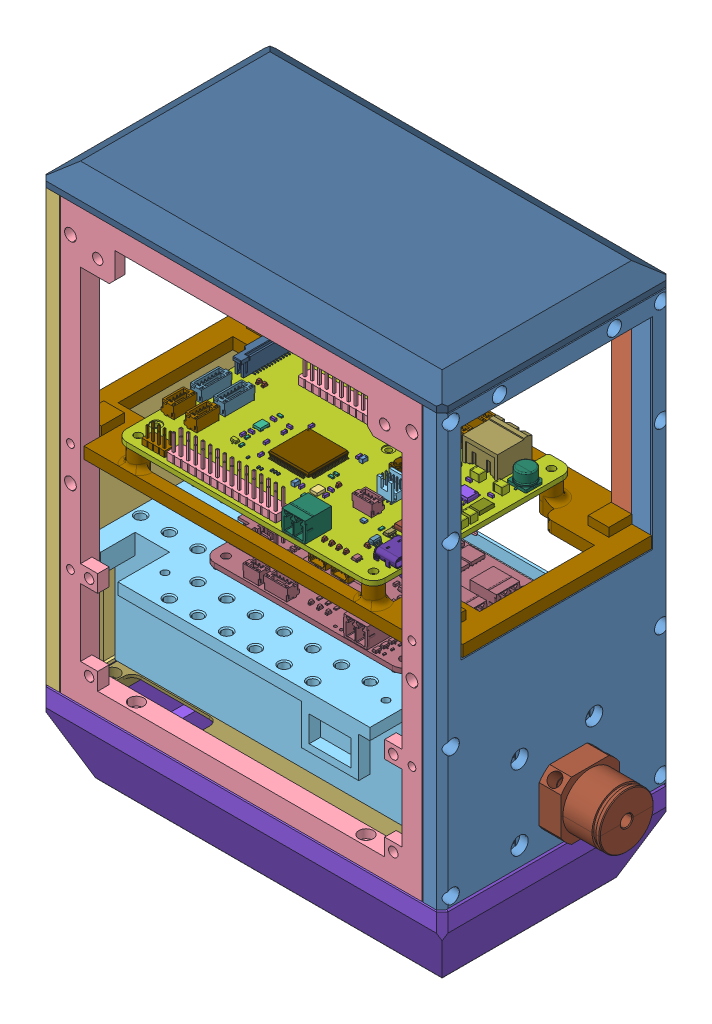
SolidWorks assembly twipr, configuration Default. Lengths in mm.
Overall size (188.64 187 80).
480 component instances, 72 part files, 48 mates.
Components (placement in the parent):
- twipr_sketch-1: twipr_sketch [Default] at origin (hidden)
- brace_left-1: brace_left [Default] at (-379.6774 202.2203 0) x (0 0 -1) z (1 0 0) size (80 150 10.2)
- brace_front-1: brace_front [Default] at (-442.6774 202.2203 -40) size (126 150 7)
- brace_right-1: brace_right [Default] at (-505.6774 202.2203 0) x (0 0 1) z (-1 0 0) size (80 150 7)
- brace_back-1: brace_back [Default] at (-442.6774 202.2203 33) size (126 150 7)
- platform_middle-1: platform_middle [Default] at (-442.7274 165.7203 0) size (126 42 78)
- banebots_4_78-1: banebots_4_78 [Default] at (-368.872 147.2203 0) x (0 0 -1) z (1 0 0) size (123.83 123.83 21.34) (hidden)
- banebots_4_78-2: banebots_4_78 [Default] at (-516.2261 147.2203 0) x (0 0 1) z (-1 0 0) size (123.83 123.83 21.34) (hidden)
- robot-hub-1: robot-hub [Default] at (-323.8774 211.7203 115.5) x (-1 0 0) z (0 1 0) size (91.46 70 13.31)
  - robot-hub.step-1: robot-hub.step [Default] at origin size (91.46 70 13.31)
    - R_0603_1608Metric.step-1: R_0603_1608Metric.step [Default] at (112.6 -91.1 1.71) x (0 1 0) z (0 0 1) size (1.6 0.8 0.45)
      - SOLID.step-1: SOLID.step [Default] at origin size (1.6 0.8 0.45)
    - C_1210_3225Metric.step-1: C_1210_3225Metric.step [Default] at (76.55 -102.85 1.71) x (-1 0 0) z (0 0 1) size (3.2 2.5 2.5)
      - SOLID-0.step-1: SOLID-0.step [Default] at origin size (3.2 2.5 2.5)
    - C_0603_1608Metric.step-1: C_0603_1608Metric.step [Default] at (132.2 -95.8 1.71) x (0 1 0) z (0 0 1) size (1.6 0.8 0.8)
      - SOLID-1.step-1: SOLID-1.step [Default] at origin size (1.6 0.8 0.8)
    - JST_GH_BM04B-GHS-TBT_1x04-1MP_P1.25mm_Vertical.step-1: JST_GH_BM04B-GHS-TBT_1x04-1MP_P1.25mm_Vertical.step [Default] at (152.6 -95.3 1.71) x (0 1 0) z (0 0 1) size (8.25 4.95 4.2)
      - SOLID-2.step-1: SOLID-2.step [Default] at origin size (8.25 4.95 4.2)
    - R_0603_1608Metric.step-2: R_0603_1608Metric.step [Default] at (107.5 -84.7687 1.71) x (0 -1 0) z (0 0 1) size (1.6 0.8 0.45)
      - SOLID.step-1: SOLID.step [Default] at origin size (1.6 0.8 0.45)
    - R_0402_1005Metric.step-1: R_0402_1005Metric.step [Default] at (123.5 -93.2 1.71) x (0 1 0) z (0 0 1) size (1 0.5 0.35)
      - SOLID-3.step-1: SOLID-3.step [Default] at origin size (1 0.5 0.35)
    - LED_0603_1608Metric.step-1: LED_0603_1608Metric.step [Default] at (88 -81.3 1.71) x (0 -1 0) z (0 0 1) size (1.6 0.8 1.1)
      - SOLID-4.step-1: SOLID-4.step [Default] at origin size (1.6 0.8 1.1)
    - R_0603_1608Metric.step-3: R_0603_1608Metric.step [Default] at (113.4 -101.6 1.71) x (-1 0 0) z (0 0 1) size (1.6 0.8 0.45)
      - SOLID.step-1: SOLID.step [Default] at origin size (1.6 0.8 0.45)
    - LTC4412ES6#TRMPBF.step-1: LTC4412ES6#TRMPBF.step [Default] at (86.1 -94.6 1.71) size (2.8 2.9 1)
      - COMPOUND.step-1: COMPOUND.step [Default] at origin size (2.8 2.9 1)
    - ws2812_2020.step-1: ws2812_2020.step [Default] at (84.3 -81.3 1.71) size (2.2 2 0.84)
      - COMPOUND-5.step-1: COMPOUND-5.step [Default] at origin size (2.2 2 0.84)
    - LED_0603_1608Metric.step-2: LED_0603_1608Metric.step [Default] at (86.1 -86.8 1.71) size (1.6 0.8 1.1)
      - SOLID-4.step-1: SOLID-4.step [Default] at origin size (1.6 0.8 1.1)
    - R_0402_1005Metric.step-2: R_0402_1005Metric.step [Default] at (133.8 -92.9 1.71) x (0 -1 0) z (0 0 1) size (1 0.5 0.35)
      - SOLID-3.step-1: SOLID-3.step [Default] at origin size (1 0.5 0.35)
    - JST_GH_BM06B-GHS-TBT_1x06-1MP_P1.25mm_Vertical.step-1: JST_GH_BM06B-GHS-TBT_1x06-1MP_P1.25mm_Vertical.step [Default] at (114 -135.2 1.71) size (10.75 4.95 4.2)
      - SOLID-6.step-1: SOLID-6.step [Default] at origin size (10.75 4.95 4.2)
    - JST_GH_BM04B-GHS-TBT_1x04-1MP_P1.25mm_Vertical.step-2: JST_GH_BM04B-GHS-TBT_1x04-1MP_P1.25mm_Vertical.step [Default] at (134.6 -135.2 1.71) size (8.25 4.95 4.2)
      - SOLID-2.step-1: SOLID-2.step [Default] at origin size (8.25 4.95 4.2)
    - C_0603_1608Metric.step-2: C_0603_1608Metric.step [Default] at (109.4 -97.4 1.71) x (-1 0 0) z (0 0 1) size (1.6 0.8 0.8)
      - SOLID-1.step-1: SOLID-1.step [Default] at origin size (1.6 0.8 0.8)
    - C_1210_3225Metric.step-2: C_1210_3225Metric.step [Default] at (87.55 -126.8 1.71) size (3.2 2.5 2.5)
      - SOLID-0.step-1: SOLID-0.step [Default] at origin size (3.2 2.5 2.5)
    - C_1210_3225Metric.step-3: C_1210_3225Metric.step [Default] at (76.55 -109.6 1.71) x (-1 0 0) z (0 0 1) size (3.2 2.5 2.5)
      - SOLID-0.step-1: SOLID-0.step [Default] at origin size (3.2 2.5 2.5)
    - R_0603_1608Metric.step-4: R_0603_1608Metric.step [Default] at (138.6 -95.5 1.71) x (0 -1 0) z (0 0 1) size (1.6 0.8 0.45)
      - SOLID.step-1: SOLID.step [Default] at origin size (1.6 0.8 0.45)
    - CP_Elec_6.3x5.2.step-1: CP_Elec_6.3x5.2.step [Default] at (77.8 -133.7 1.71) x (0 1 0) z (0 0 1) size (10.2 10.92 5.2)
      - SOLID-7.step-1: SOLID-7.step [Default] at origin size (10.2 10.92 5.2)
    - R_0402_1005Metric.step-3: R_0402_1005Metric.step [Default] at (127.9 -91.7 1.71) x (0 -1 0) z (0 0 1) size (1 0.5 0.35)
      - SOLID-3.step-1: SOLID-3.step [Default] at origin size (1 0.5 0.35)
    - R_0603_1608Metric.step-5: R_0603_1608Metric.step [Default] at (104.2 -119.8 1.71) size (1.6 0.8 0.45)
      - SOLID.step-1: SOLID.step [Default] at origin size (1.6 0.8 0.45)
    - C_0603_1608Metric.step-3: C_0603_1608Metric.step [Default] at (132 -113.2 1.71) x (0 -1 0) z (0 0 1) size (1.6 0.8 0.8)
      - SOLID-1.step-1: SOLID-1.step [Default] at origin size (1.6 0.8 0.8)
    - JST_GH_BM04B-GHS-TBT_1x04-1MP_P1.25mm_Vertical.step-3: JST_GH_BM04B-GHS-TBT_1x04-1MP_P1.25mm_Vertical.step [Default] at (97.4 -125.1 1.71) size (8.25 4.95 4.2)
      - SOLID-2.step-1: SOLID-2.step [Default] at origin size (8.25 4.95 4.2)
    - C_0603_1608Metric.step-4: C_0603_1608Metric.step [Default] at (87.8 -117.65 1.71) x (0 -1 0) z (0 0 1) size (1.6 0.8 0.8)
      - SOLID-1.step-1: SOLID-1.step [Default] at origin size (1.6 0.8 0.8)
    - JST_GH_BM06B-GHS-TBT_1x06-1MP_P1.25mm_Vertical.step-2: JST_GH_BM06B-GHS-TBT_1x06-1MP_P1.25mm_Vertical.step [Default] at (160.6 -106.3 1.71) x (0 1 0) z (0 0 1) size (10.75 4.95 4.2)
      - SOLID-6.step-1: SOLID-6.step [Default] at origin size (10.75 4.95 4.2)
    - JST_GH_BM02B-GHS-TBT_1x02-1MP_P1.25mm_Vertical.step-1: JST_GH_BM02B-GHS-TBT_1x02-1MP_P1.25mm_Vertical.step [Default] at (152.5 -143.25 1.71) size (5.75 4.95 4.2)
      - SOLID-8.step-1: SOLID-8.step [Default] at origin size (5.75 4.95 4.2)
    - USB4105-GF-A.step-1: USB4105-GF-A.step [Default] at (76.635 -88.9375 1.71) x (0 -1 0) z (-1 0 0) size (9.58 4.16 7.71)
      - COMPOUND-9.step-1: COMPOUND-9.step [Default] at origin size (9.58 4.16 7.71)
    - JST_GH_BM04B-GHS-TBT_1x04-1MP_P1.25mm_Vertical.step-4: JST_GH_BM04B-GHS-TBT_1x04-1MP_P1.25mm_Vertical.step [Default] at (160.6 -95.3 1.71) x (0 1 0) z (0 0 1) size (8.25 4.95 4.2)
      - SOLID-2.step-1: SOLID-2.step [Default] at origin size (8.25 4.95 4.2)
    - 4341x30258x6 (rev1).step-1: 4341x30258x6 (rev1).step [Default] at (104.2 -116 1.71) x (1 0 0) z (0 -1 0) size (3.2 2.5 4.6)
      - COMPOUND-10.step-1: COMPOUND-10.step [Default] at origin size (3.2 2.5 4.6)
    - JST_GH_BM04B-GHS-TBT_1x04-1MP_P1.25mm_Vertical.step-5: JST_GH_BM04B-GHS-TBT_1x04-1MP_P1.25mm_Vertical.step [Default] at (103.2 -143.2 1.71) size (8.25 4.95 4.2)
      - SOLID-2.step-1: SOLID-2.step [Default] at origin size (8.25 4.95 4.2)
    - C_0805_2012Metric.step-1: C_0805_2012Metric.step [Default] at (112.7 -112 1.71) x (0 1 0) z (0 0 1) size (2 1.25 1.25)
      - SOLID-11.step-1: SOLID-11.step [Default] at origin size (2 1.25 1.25)
    - CUI_DEVICES_CMT-7525-80-SMT-TR.step-1: CUI_DEVICES_CMT-7525-80-SMT-TR.step [Default] at (97.3 -115.8 1.71) x (1 0 0) z (0 -1 0) size (7.5 2.5 7.5)
      - COMPOUND-12.step-1: COMPOUND-12.step [Default] at origin size (7.5 2.5 7.5)
    - BMX160.step-1: BMX160.step [Default] at (111.35 -94.75 1.71) x (0 -1 0) z (-1 0 0) size (3 1 2.5)
      - COMPOUND-13.step-1: COMPOUND-13.step [Default] at origin size (3 1 2.5)
    - PinHeader_2x15_P2.54mm_Vertical.step-1: PinHeader_2x15_P2.54mm_Vertical.step [Default] at (110.525 -127.545 1.71) x (0 1 0) z (0 0 1) size (5.08 38.1 11.54)
      - SOLID-14.step-1: SOLID-14.step [Default] at origin size (5.08 38.1 11.54)
    - C_0603_1608Metric.step-5: C_0603_1608Metric.step [Default] at (115.5 -93.3 1.71) x (0 1 0) z (0 0 1) size (1.6 0.8 0.8)
      - SOLID-1.step-1: SOLID-1.step [Default] at origin size (1.6 0.8 0.8)
    - JST_GH_BM02B-GHS-TBT_1x02-1MP_P1.25mm_Vertical.step-2: JST_GH_BM02B-GHS-TBT_1x02-1MP_P1.25mm_Vertical.step [Default] at (152.5 -135.25 1.71) size (5.75 4.95 4.2)
      - SOLID-8.step-1: SOLID-8.step [Default] at origin size (5.75 4.95 4.2)
    - FTSH-105-01-L-DV-K.step-1: FTSH-105-01-L-DV-K.step [Default] at (97.4 -106.5 2.21) x (-1 0 0) z (0 1 0) size (6.35 6.12 5.84)
      - COMPOUND-15.step-1: COMPOUND-15.step [Default] at origin size (6.35 6.12 5.84)
    - JST_GH_BM04B-GHS-TBT_1x04-1MP_P1.25mm_Vertical.step-6: JST_GH_BM04B-GHS-TBT_1x04-1MP_P1.25mm_Vertical.step [Default] at (103.2 -135.2 1.71) size (8.25 4.95 4.2)
      - SOLID-2.step-1: SOLID-2.step [Default] at origin size (8.25 4.95 4.2)
    - C_0603_1608Metric.step-6: C_0603_1608Metric.step [Default] at (141.5 -98.8 1.71) x (0 1 0) z (0 0 1) size (1.6 0.8 0.8)
      - SOLID-1.step-1: SOLID-1.step [Default] at origin size (1.6 0.8 0.8)
    - ECS-250-18-33B-CKY-TR.step-1: ECS-250-18-33B-CKY-TR.step [Default] at (140.9 -104.6 1.71) x (0 1 0) z (0 0 1) size (3.38 2.78 0.9)
      - COMPOUND-16.step-1: COMPOUND-16.step [Default] at origin size (3.38 2.78 0.9)
    - C_0603_1608Metric.step-7: C_0603_1608Metric.step [Default] at (114.5 -112.3 1.71) x (0 1 0) z (0 0 1) size (1.6 0.8 0.8)
      - SOLID-1.step-1: SOLID-1.step [Default] at origin size (1.6 0.8 0.8)
    - JST_GH_BM06B-GHS-TBT_1x06-1MP_P1.25mm_Vertical.step-3: JST_GH_BM06B-GHS-TBT_1x06-1MP_P1.25mm_Vertical.step [Default] at (113.95 -143.2 1.71) size (10.75 4.95 4.2)
      - SOLID-6.step-1: SOLID-6.step [Default] at origin size (10.75 4.95 4.2)
    - C_0603_1608Metric.step-8: C_0603_1608Metric.step [Default] at (134.9 -106.6 1.71) x (0 -1 0) z (0 0 1) size (1.6 0.8 0.8)
      - SOLID-1.step-1: SOLID-1.step [Default] at origin size (1.6 0.8 0.8)
    - SOT-323_SC-70.step-1: SOT-323_SC-70.step [Default] at (140.9 -95.4 1.71) x (0 1 0) z (0 0 1) size (2 2 1.05)
      - SOLID-17.step-1: SOLID-17.step [Default] at origin size (2 2 1.05)
    - LED_0603_1608Metric.step-3: LED_0603_1608Metric.step [Default] at (109.4 -100.1 1.71) x (0 -1 0) z (0 0 1) size (1.6 0.8 1.1)
      - SOLID-4.step-1: SOLID-4.step [Default] at origin size (1.6 0.8 1.1)
    - LMR33630ADDA.step-1: LMR33630ADDA.step [Default] at (84.05 -119.1 1.71) x (0 1 0) z (0 0 1) size (6 4.9 1.7)
      - COMPOUND-18.step-1: COMPOUND-18.step [Default] at origin size (6 4.9 1.7)
    - C_0603_1608Metric.step-9: C_0603_1608Metric.step [Default] at (88.3 -124.4 1.71) size (1.6 0.8 0.8)
      - SOLID-1.step-1: SOLID-1.step [Default] at origin size (1.6 0.8 0.8)
    - C_0603_1608Metric.step-10: C_0603_1608Metric.step [Default] at (140.8 -101.1 1.71) size (1.6 0.8 0.8)
      - SOLID-1.step-1: SOLID-1.step [Default] at origin size (1.6 0.8 0.8)
    - PinHeader_2x04_P2.00mm_Vertical.step-1: PinHeader_2x04_P2.00mm_Vertical.step [Default] at (149.4 -81.4 1.71) x (0 1 0) z (0 0 1) size (4 8 8.8)
      - SOLID-19.step-1: SOLID-19.step [Default] at origin size (4 8 8.8)
    - 1-1734248-5.step-1: 1-1734248-5.step [Default] at (159.98 -126.3 6.21) x (0 1 0) z (0 0 1) size (22.4 4.85 5.68)
      - SOLID-20.step-1: SOLID-20.step [Default] at origin size (22.4 4.85 5.68)
    - IS25LP032D-JNLA3-TR.step-1: IS25LP032D-JNLA3-TR.step [Default] at (84.9 -99.3 1.71) x (-1 0 0) z (0 0 1) size (6 4.9 1.75)
      - COMPOUND-21.step-1: COMPOUND-21.step [Default] at origin size (6 4.9 1.75)
    - 691313510002.step-1: 691313510002.step [Default] at (89.3 -135.2 5.71) x (-1 0 0) z (0 -1 0) size (12.16 12 12)
      - COMPOUND-22.step-1: COMPOUND-22.step [Default] at origin size (12.16 12 12)
    - LED_0603_1608Metric.step-4: LED_0603_1608Metric.step [Default] at (93 -81.3 1.71) x (0 -1 0) z (0 0 1) size (1.6 0.8 1.1)
      - SOLID-4.step-1: SOLID-4.step [Default] at origin size (1.6 0.8 1.1)
    - JST_GH_BM04B-GHS-TBT_1x04-1MP_P1.25mm_Vertical.step-7: JST_GH_BM04B-GHS-TBT_1x04-1MP_P1.25mm_Vertical.step [Default] at (124.95 -135.2 1.71) size (8.25 4.95 4.2)
      - SOLID-2.step-1: SOLID-2.step [Default] at origin size (8.25 4.95 4.2)
    - LED_0603_1608Metric.step-5: LED_0603_1608Metric.step [Default] at (154.5 -117.4 1.71) x (0 -1 0) z (0 0 1) size (1.6 0.8 1.1)
      - SOLID-4.step-1: SOLID-4.step [Default] at origin size (1.6 0.8 1.1)
    - JST_GH_BM03B-GHS-TBT_1x03-1MP_P1.25mm_Vertical.step-1: JST_GH_BM03B-GHS-TBT_1x03-1MP_P1.25mm_Vertical.step [Default] at (97.4 -98.7 1.71) size (7 4.95 4.2)
      - SOLID-23.step-1: SOLID-23.step [Default] at origin size (7 4.95 4.2)
    - C_0603_1608Metric.step-11: C_0603_1608Metric.step [Default] at (108.6 -94.8 1.71) x (0 -1 0) z (0 0 1) size (1.6 0.8 0.8)
      - SOLID-1.step-1: SOLID-1.step [Default] at origin size (1.6 0.8 0.8)
    - R_0603_1608Metric.step-6: R_0603_1608Metric.step [Default] at (113.4 -103.2 1.71) size (1.6 0.8 0.45)
      - SOLID.step-1: SOLID.step [Default] at origin size (1.6 0.8 0.45)
    - LED_0603_1608Metric.step-6: LED_0603_1608Metric.step [Default] at (95.5 -81.3 1.71) x (0 -1 0) z (0 0 1) size (1.6 0.8 1.1)
      - SOLID-4.step-1: SOLID-4.step [Default] at origin size (1.6 0.8 1.1)
    - R_0402_1005Metric.step-4: R_0402_1005Metric.step [Default] at (125.7 -93.2 1.71) x (0 -1 0) z (0 0 1) size (1 0.5 0.35)
      - SOLID-3.step-1: SOLID-3.step [Default] at origin size (1 0.5 0.35)
    - SOT-23-6.step-1: SOT-23-6.step [Default] at (86.1 -89.45 1.71) x (-1 0 0) z (0 0 1) size (2.8 2.9 1.55)
      - SOLID-24.step-1: SOLID-24.step [Default] at origin size (2.8 2.9 1.55)
    - R_0603_1608Metric.step-7: R_0603_1608Metric.step [Default] at (89.3 -117.65 1.71) x (0 -1 0) z (0 0 1) size (1.6 0.8 0.45)
      - SOLID.step-1: SOLID.step [Default] at origin size (1.6 0.8 0.45)
    - R_0603_1608Metric.step-8: R_0603_1608Metric.step [Default] at (92.3 -111.9 1.71) x (0 1 0) z (0 0 1) size (1.6 0.8 0.45)
      - SOLID.step-1: SOLID.step [Default] at origin size (1.6 0.8 0.45)
    - R_0603_1608Metric.step-9: R_0603_1608Metric.step [Default] at (88.55 -115.4 1.71) size (1.6 0.8 0.45)
      - SOLID.step-1: SOLID.step [Default] at origin size (1.6 0.8 0.45)
    - 691322110002.step-1: 691322110002.step [Default] at (101.9 -81.4 5.21) x (-1 0 0) z (0 1 0) size (8.4 10.7 9.2)
      - COMPOUND-25.step-1: COMPOUND-25.step [Default] at origin size (8.4 10.7 9.2)
    - LED_0603_1608Metric.step-7: LED_0603_1608Metric.step [Default] at (90.5 -81.3 1.71) x (0 -1 0) z (0 0 1) size (1.6 0.8 1.1)
      - SOLID-4.step-1: SOLID-4.step [Default] at origin size (1.6 0.8 1.1)
    - JST_GH_BM06B-GHS-TBT_1x06-1MP_P1.25mm_Vertical.step-4: JST_GH_BM06B-GHS-TBT_1x06-1MP_P1.25mm_Vertical.step [Default] at (152.6 -106.3 1.71) x (0 1 0) z (0 0 1) size (10.75 4.95 4.2)
      - SOLID-6.step-1: SOLID-6.step [Default] at origin size (10.75 4.95 4.2)
    - R_0603_1608Metric.step-10: R_0603_1608Metric.step [Default] at (140 -98.8 1.71) x (0 -1 0) z (0 0 1) size (1.6 0.8 0.45)
      - SOLID.step-1: SOLID.step [Default] at origin size (1.6 0.8 0.45)
    - C_1210_3225Metric.step-4: C_1210_3225Metric.step [Default] at (79.6 -126.9 1.71) x (-1 0 0) z (0 0 1) size (3.2 2.5 2.5)
      - SOLID-0.step-1: SOLID-0.step [Default] at origin size (3.2 2.5 2.5)
    - JST_GH_BM04B-GHS-TBT_1x04-1MP_P1.25mm_Vertical.step-8: JST_GH_BM04B-GHS-TBT_1x04-1MP_P1.25mm_Vertical.step [Default] at (134.6 -143.2 1.71) size (8.25 4.95 4.2)
      - SOLID-2.step-1: SOLID-2.step [Default] at origin size (8.25 4.95 4.2)
    - PDS760-13.step-1: PDS760-13.step [Default] at (77.99 -118.49 1.71) x (1 0 0) z (0 -1 0) size (3.9 1.05 6.4)
      - COMPOUND-26.step-1: COMPOUND-26.step [Default] at origin size (3.9 1.05 6.4)
    - PinHeader_2x15_P2.54mm_Vertical.step-2: PinHeader_2x15_P2.54mm_Vertical.step [Default] at (110.525 -81.825 1.71) x (0 1 0) z (0 0 1) size (5.08 38.1 11.54)
      - SOLID-14.step-1: SOLID-14.step [Default] at origin size (5.08 38.1 11.54)
    - LED_0603_1608Metric.step-8: LED_0603_1608Metric.step [Default] at (96.8 -143.9 1.71) x (0 -1 0) z (0 0 1) size (1.6 0.8 1.1)
      - SOLID-4.step-1: SOLID-4.step [Default] at origin size (1.6 0.8 1.1)
    - 744325.step-1: 744325.step [Default] at (84.55 -108.35 1.71) x (-1 0 0) z (0 0 1) size (10.74 11.01 5.01)
      - COMPOUND-27.step-1: COMPOUND-27.step [Default] at origin size (10.74 11.01 5.01)
    - R_0603_1608Metric.step-11: R_0603_1608Metric.step [Default] at (111.05 -91.05 1.71) x (0 1 0) z (0 0 1) size (1.6 0.8 0.45)
      - SOLID.step-1: SOLID.step [Default] at origin size (1.6 0.8 0.45)
    - C_0603_1608Metric.step-12: C_0603_1608Metric.step [Default] at (140.75 -108.7 1.71) x (-1 0 0) z (0 0 1) size (1.6 0.8 0.8)
      - SOLID-1.step-1: SOLID-1.step [Default] at origin size (1.6 0.8 0.8)
    - C_0603_1608Metric.step-13: C_0603_1608Metric.step [Default] at (135.6 -109.2 1.71) size (1.6 0.8 0.8)
      - SOLID-1.step-1: SOLID-1.step [Default] at origin size (1.6 0.8 0.8)
    - R_0603_1608Metric.step-12: R_0603_1608Metric.step [Default] at (140.7 -111 1.71) size (1.6 0.8 0.45)
      - SOLID.step-1: SOLID.step [Default] at origin size (1.6 0.8 0.45)
    - LQFP-100_14x14mm_P0.5mm.step-1: LQFP-100_14x14mm_P0.5mm.step [Default] at (124 -104.2 1.71) x (-1 0 0) z (0 0 1) size (16 16 1.5)
      - SOLID-28.step-1: SOLID-28.step [Default] at origin size (16 16 1.5)
    - R_0603_1608Metric.step-13: R_0603_1608Metric.step [Default] at (87.8 -120.65 1.71) x (0 1 0) z (0 0 1) size (1.6 0.8 0.45)
      - SOLID.step-1: SOLID.step [Default] at origin size (1.6 0.8 0.45)
    - C_1210_3225Metric.step-5: C_1210_3225Metric.step [Default] at (76.55 -112.85 1.71) x (-1 0 0) z (0 0 1) size (3.2 2.5 2.5)
      - SOLID-0.step-1: SOLID-0.step [Default] at origin size (3.2 2.5 2.5)
    - R_0402_1005Metric.step-5: R_0402_1005Metric.step [Default] at (124.6 -93.2 1.71) x (0 1 0) z (0 0 1) size (1 0.5 0.35)
      - SOLID-3.step-1: SOLID-3.step [Default] at origin size (1 0.5 0.35)
    - SOT-563.step-1: SOT-563.step [Default] at (94.4 -93.9 1.71) x (0 -1 0) z (0 0 1) size (1.6 1.6 0.63)
      - SOLID-29.step-1: SOLID-29.step [Default] at origin size (1.6 1.6 0.63)
    - JST_GH_BM04B-GHS-TBT_1x04-1MP_P1.25mm_Vertical.step-9: JST_GH_BM04B-GHS-TBT_1x04-1MP_P1.25mm_Vertical.step [Default] at (144.225 -143.2344 1.71) size (8.25 4.95 4.2)
      - SOLID-2.step-1: SOLID-2.step [Default] at origin size (8.25 4.95 4.2)
    - C_1210_3225Metric.step-6: C_1210_3225Metric.step [Default] at (76.55 -106.35 1.71) x (-1 0 0) z (0 0 1) size (3.2 2.5 2.5)
      - SOLID-0.step-1: SOLID-0.step [Default] at origin size (3.2 2.5 2.5)
    - C_0603_1608Metric.step-14: C_0603_1608Metric.step [Default] at (79.8 -123.6 1.71) x (-1 0 0) z (0 0 1) size (1.6 0.8 0.8)
      - SOLID-1.step-1: SOLID-1.step [Default] at origin size (1.6 0.8 0.8)
    - R_0402_1005Metric.step-6: R_0402_1005Metric.step [Default] at (129 -91.7 1.71) x (0 -1 0) z (0 0 1) size (1 0.5 0.35)
      - SOLID-3.step-1: SOLID-3.step [Default] at origin size (1 0.5 0.35)
    - LED_0603_1608Metric.step-9: LED_0603_1608Metric.step [Default] at (107.5 -81.6688 1.71) x (0 -1 0) z (0 0 1) size (1.6 0.8 1.1)
      - SOLID-4.step-1: SOLID-4.step [Default] at origin size (1.6 0.8 1.1)
    - JST_GH_BM04B-GHS-TBT_1x04-1MP_P1.25mm_Vertical.step-10: JST_GH_BM04B-GHS-TBT_1x04-1MP_P1.25mm_Vertical.step [Default] at (124.95 -143.2 1.71) size (8.25 4.95 4.2)
      - SOLID-2.step-1: SOLID-2.step [Default] at origin size (8.25 4.95 4.2)
    - LED_0603_1608Metric.step-10: LED_0603_1608Metric.step [Default] at (152.6 -117.4 1.71) x (0 -1 0) z (0 0 1) size (1.6 0.8 1.1)
      - SOLID-4.step-1: SOLID-4.step [Default] at origin size (1.6 0.8 1.1)
    - C_0805_2012Metric.step-2: C_0805_2012Metric.step [Default] at (117.4 -93.1 1.71) x (0 -1 0) z (0 0 1) size (2 1.25 1.25)
      - SOLID-11.step-1: SOLID-11.step [Default] at origin size (2 1.25 1.25)
    - C_0603_1608Metric.step-15: C_0603_1608Metric.step [Default] at (135 -100.5 1.71) x (0 -1 0) z (0 0 1) size (1.6 0.8 0.8)
      - SOLID-1.step-1: SOLID-1.step [Default] at origin size (1.6 0.8 0.8)
    - R_0603_1608Metric.step-14: R_0603_1608Metric.step [Default] at (89 -94.6 1.71) x (0 -1 0) z (0 0 1) size (1.6 0.8 0.45)
      - SOLID.step-1: SOLID.step [Default] at origin size (1.6 0.8 0.45)
    - JST_GH_BM04B-GHS-TBT_1x04-1MP_P1.25mm_Vertical.step-11: JST_GH_BM04B-GHS-TBT_1x04-1MP_P1.25mm_Vertical.step [Default] at (144.225 -135.2344 1.71) size (8.25 4.95 4.2)
      - SOLID-2.step-1: SOLID-2.step [Default] at origin size (8.25 4.95 4.2)
    - R_0603_1608Metric.step-15: R_0603_1608Metric.step [Default] at (99.6 -129.6 -0.05) x (0 1 0) z (0 0 -1) size (1.6 0.8 0.45)
      - SOLID.step-1: SOLID.step [Default] at origin size (1.6 0.8 0.45)
    - C_0603_1608Metric.step-16: C_0603_1608Metric.step [Default] at (131.9625 -133.35 -0.05) x (0 1 0) z (0 0 -1) size (1.6 0.8 0.8)
      - SOLID-1.step-1: SOLID-1.step [Default] at origin size (1.6 0.8 0.8)
    - R_0603_1608Metric.step-16: R_0603_1608Metric.step [Default] at (119.6 -120.9 -0.05) x (-1 0 0) z (0 0 -1) size (1.6 0.8 0.45)
      - SOLID.step-1: SOLID.step [Default] at origin size (1.6 0.8 0.45)
    - R_0402_1005Metric.step-7: R_0402_1005Metric.step [Default] at (97.7 -85.3 -0.05) x (0 1 0) z (0 0 -1) size (1 0.5 0.35)
      - SOLID-3.step-1: SOLID-3.step [Default] at origin size (1 0.5 0.35)
    - C_0805_2012Metric.step-3: C_0805_2012Metric.step [Default] at (92.5 -98.9 -0.05) x (0 -1 0) z (0 0 -1) size (2 1.25 1.25)
      - SOLID-11.step-1: SOLID-11.step [Default] at origin size (2 1.25 1.25)
    - R_0402_1005Metric.step-8: R_0402_1005Metric.step [Default] at (91.95 -90.35 -0.05) x (-1 0 0) z (0 0 -1) size (1 0.5 0.35)
      - SOLID-3.step-1: SOLID-3.step [Default] at origin size (1 0.5 0.35)
    - MSOP-10_3x3mm_P0.5mm.step-1: MSOP-10_3x3mm_P0.5mm.step [Default] at (111.8 -114.8 -0.05) x (-1 0 0) z (0 0 -1) size (4.9 3 0.95)
      - SOLID-30.step-1: SOLID-30.step [Default] at origin size (4.9 3 0.95)
    - STM32G031G6U6.step-1: STM32G031G6U6.step [Default] at (95.6 -89.05 -0.05) x (0 1 0) z (0 0 -1) size (4.1 4.1 0.6)
      - COMPOUND-31.step-1: COMPOUND-31.step [Default] at origin size (4.1 4.1 0.6)
    - R_0603_1608Metric.step-17: R_0603_1608Metric.step [Default] at (137.5 -144 -0.05) x (0 -1 0) z (0 0 -1) size (1.6 0.8 0.45)
      - SOLID.step-1: SOLID.step [Default] at origin size (1.6 0.8 0.45)
    - R_0603_1608Metric.step-18: R_0603_1608Metric.step [Default] at (137.4625 -136.35 -0.05) x (0 -1 0) z (0 0 -1) size (1.6 0.8 0.45)
      - SOLID.step-1: SOLID.step [Default] at origin size (1.6 0.8 0.45)
    - C_0603_1608Metric.step-17: C_0603_1608Metric.step [Default] at (139 -140.9 -0.05) x (0 1 0) z (0 0 -1) size (1.6 0.8 0.8)
      - SOLID-1.step-1: SOLID-1.step [Default] at origin size (1.6 0.8 0.8)
    - R_0603_1608Metric.step-19: R_0603_1608Metric.step [Default] at (97.5 -137.2 -0.05) x (0 1 0) z (0 0 -1) size (1.6 0.8 0.45)
      - SOLID.step-1: SOLID.step [Default] at origin size (1.6 0.8 0.45)
    - R_0603_1608Metric.step-20: R_0603_1608Metric.step [Default] at (117.6 -113.8 -0.05) x (-1 0 0) z (0 0 -1) size (1.6 0.8 0.45)
      - SOLID.step-1: SOLID.step [Default] at origin size (1.6 0.8 0.45)
    - R_0603_1608Metric.step-21: R_0603_1608Metric.step [Default] at (156.7 -115 -0.05) x (0 1 0) z (0 0 -1) size (1.6 0.8 0.45)
      - SOLID.step-1: SOLID.step [Default] at origin size (1.6 0.8 0.45)
    - C_0603_1608Metric.step-18: C_0603_1608Metric.step [Default] at (126.85 -136.2 -0.05) x (0 1 0) z (0 0 -1) size (1.6 0.8 0.8)
      - SOLID-1.step-1: SOLID-1.step [Default] at origin size (1.6 0.8 0.8)
    - R_0603_1608Metric.step-22: R_0603_1608Metric.step [Default] at (97.9 -129.6 -0.05) x (0 1 0) z (0 0 -1) size (1.6 0.8 0.45)
      - SOLID.step-1: SOLID.step [Default] at origin size (1.6 0.8 0.45)
    - C_0805_2012Metric.step-4: C_0805_2012Metric.step [Default] at (99.15 -100.9 -0.05) x (0 1 0) z (0 0 -1) size (2 1.25 1.25)
      - SOLID-11.step-1: SOLID-11.step [Default] at origin size (2 1.25 1.25)
    - R_0402_1005Metric.step-9: R_0402_1005Metric.step [Default] at (88.15 -88.95 -0.05) x (0 -1 0) z (0 0 -1) size (1 0.5 0.35)
      - SOLID-3.step-1: SOLID-3.step [Default] at origin size (1 0.5 0.35)
    - R_0603_1608Metric.step-23: R_0603_1608Metric.step [Default] at (96.3 -129.6 -0.05) x (0 1 0) z (0 0 -1) size (1.6 0.8 0.45)
      - SOLID.step-1: SOLID.step [Default] at origin size (1.6 0.8 0.45)
    - R_0402_1005Metric.step-10: R_0402_1005Metric.step [Default] at (91.96 -86.35 -0.05) x (-1 0 0) z (0 0 -1) size (1 0.5 0.35)
      - SOLID-3.step-1: SOLID-3.step [Default] at origin size (1 0.5 0.35)
    - Fuse_1206_3216Metric.step-1: Fuse_1206_3216Metric.step [Default] at (82.7 -138.7 -0.05) x (-1 0 0) z (0 0 -1) size (3.2 1.6 0.55)
      - SOLID-32.step-1: SOLID-32.step [Default] at origin size (3.2 1.6 0.55)
    - R_0603_1608Metric.step-24: R_0603_1608Metric.step [Default] at (125.4 -130.4 -0.05) x (0 -1 0) z (0 0 -1) size (1.6 0.8 0.45)
      - SOLID.step-1: SOLID.step [Default] at origin size (1.6 0.8 0.45)
    - R_0603_1608Metric.step-25: R_0603_1608Metric.step [Default] at (144.7 -142.2 -0.05) x (1 0 0) z (0 0 -1) size (1.6 0.8 0.45)
      - SOLID.step-1: SOLID.step [Default] at origin size (1.6 0.8 0.45)
    - R_0603_1608Metric.step-26: R_0603_1608Metric.step [Default] at (151.2 -84.3 -0.05) x (0 1 0) z (0 0 -1) size (1.6 0.8 0.45)
      - SOLID.step-1: SOLID.step [Default] at origin size (1.6 0.8 0.45)
    - R_0603_1608Metric.step-27: R_0603_1608Metric.step [Default] at (96 -137.2 -0.05) x (0 1 0) z (0 0 -1) size (1.6 0.8 0.45)
      - SOLID.step-1: SOLID.step [Default] at origin size (1.6 0.8 0.45)
    - R_0603_1608Metric.step-28: R_0603_1608Metric.step [Default] at (104.5 -106.1 -0.05) x (-1 0 0) z (0 0 -1) size (1.6 0.8 0.45)
      - SOLID.step-1: SOLID.step [Default] at origin size (1.6 0.8 0.45)
    - DF40C-100DS.step-1: DF40C-100DS.step [Default] at (144.62 -86.64 -0.05) x (0 -1 0) z (1 0 0) size (3.38 1.45 22.6)
      - SOLID-33.step-1: SOLID-33.step [Default] at origin size (3.38 1.45 22.6)
    - DF40C-100DS.step-2: DF40C-100DS.step [Default] at (144.62 -120.56 -0.05) x (0 -1 0) z (1 0 0) size (3.38 1.45 22.6)
      - SOLID-33.step-1: SOLID-33.step [Default] at origin size (3.38 1.45 22.6)
    - R_0603_1608Metric.step-29: R_0603_1608Metric.step [Default] at (96.8 -143.9 -0.05) x (0 -1 0) z (0 0 -1) size (1.6 0.8 0.45)
      - SOLID.step-1: SOLID.step [Default] at origin size (1.6 0.8 0.45)
    - C_0603_1608Metric.step-19: C_0603_1608Metric.step [Default] at (137.4625 -133.3 -0.05) x (0 1 0) z (0 0 -1) size (1.6 0.8 0.8)
      - SOLID-1.step-1: SOLID-1.step [Default] at origin size (1.6 0.8 0.8)
    - R_0603_1608Metric.step-30: R_0603_1608Metric.step [Default] at (92.9 -93.2 -0.05) x (0 -1 0) z (0 0 -1) size (1.6 0.8 0.45)
      - SOLID.step-1: SOLID.step [Default] at origin size (1.6 0.8 0.45)
    - C_0805_2012Metric.step-5: C_0805_2012Metric.step [Default] at (101.6 -119.9 -0.05) x (0 -1 0) z (0 0 -1) size (2 1.25 1.25)
      - SOLID-11.step-1: SOLID-11.step [Default] at origin size (2 1.25 1.25)
    - MC74VHC1G14DTT1G.step-1: MC74VHC1G14DTT1G.step [Default] at (157.4 -110.9 -0.05) x (0 -1 0) z (0 0 -1) size (2.75 3 1.1)
      - COMPOUND-34.step-1: COMPOUND-34.step [Default] at origin size (2.75 3 1.1)
    - R_0603_1608Metric.step-31: R_0603_1608Metric.step [Default] at (158.3 -115 -0.05) x (0 1 0) z (0 0 -1) size (1.6 0.8 0.45)
      - SOLID.step-1: SOLID.step [Default] at origin size (1.6 0.8 0.45)
    - C_0603_1608Metric.step-20: C_0603_1608Metric.step [Default] at (88.4 -93.2 -0.05) x (0 -1 0) z (0 0 -1) size (1.6 0.8 0.8)
      - SOLID-1.step-1: SOLID-1.step [Default] at origin size (1.6 0.8 0.8)
    - 9774030151 (rev1).step-1: 9774030151 (rev1).step [Default] at (160 -87.1 -0.05) x (-1 0 0) z (0 0 -1) size (5.1 5.89 4.4)
      - SOLID-35.step-1: SOLID-35.step [Default] at origin size (5.1 5.89 4.4)
    - D_SOD-323F.step-1: D_SOD-323F.step [Default] at (96.1 -113.45 -0.05) x (-1 0 0) z (0 0 -1) size (2.5 1.25 0.73)
      - SOLID-36.step-1: SOLID-36.step [Default] at origin size (2.5 1.25 0.73)
    - SM04B-SRSS-TB_dark.step-1: SM04B-SRSS-TB_dark.step [Default] at (86.2 -81 0.2) x (1 0 0) z (0 1 0) size (6 2.96 4.95)
      - SOLID-37.step-1: SOLID-37.step [Default] at origin size (6 2.96 4.95)
    - 9774030151 (rev1).step-2: 9774030151 (rev1).step [Default] at (112 -120.1 -0.05) x (-1 0 0) z (0 0 -1) size (5.1 5.89 4.4)
      - SOLID-35.step-1: SOLID-35.step [Default] at origin size (5.1 5.89 4.4)
    - M24512-DFDW6TP.step-1: M24512-DFDW6TP.step [Default] at (121.95 -135.9 -0.05) x (1 0 0) z (0 0 -1) size (6.4 3 1.2)
      - COMPOUND-38.step-1: COMPOUND-38.step [Default] at origin size (6.4 3 1.2)
    - C_0603_1608Metric.step-21: C_0603_1608Metric.step [Default] at (126.8 -141.9 -0.05) x (0 1 0) z (0 0 -1) size (1.6 0.8 0.8)
      - SOLID-1.step-1: SOLID-1.step [Default] at origin size (1.6 0.8 0.8)
    - IRF7319TRPBF.step-1: IRF7319TRPBF.step [Default] at (152.8 -137.5 -0.05) x (0 -1 0) z (0 0 -1) size (6 4.9 1.75)
      - COMPOUND-39.step-1: COMPOUND-39.step [Default] at origin size (6 4.9 1.75)
    - SX1508BIULTRT.step-1: SX1508BIULTRT.step [Default] at (120.1 -86 -0.05) x (-1 0 0) z (0 0 -1) size (3.1 3.1 0.6)
      - COMPOUND-40.step-1: COMPOUND-40.step [Default] at origin size (3.1 3.1 0.6)
    - R_0603_1608Metric.step-32: R_0603_1608Metric.step [Default] at (147.2 -130.6 -0.05) x (0 1 0) z (0 0 -1) size (1.6 0.8 0.45)
      - SOLID.step-1: SOLID.step [Default] at origin size (1.6 0.8 0.45)
    - LTC4365CTS8#TRMPBF.step-1: LTC4365CTS8#TRMPBF.step [Default] at (91.3 -135.6 -0.05) x (-1 0 0) z (0 0 -1) size (2.8 2.9 1)
      - COMPOUND-41.step-1: COMPOUND-41.step [Default] at origin size (2.8 2.9 1)
    - C_0603_1608Metric.step-22: C_0603_1608Metric.step [Default] at (106.5 -133.3 -0.05) x (0 -1 0) z (0 0 -1) size (1.6 0.8 0.8)
      - SOLID-1.step-1: SOLID-1.step [Default] at origin size (1.6 0.8 0.8)
    - SOT-323_SC-70.step-2: SOT-323_SC-70.step [Default] at (92.8 -112.95 -0.05) x (0 -1 0) z (0 0 -1) size (2 2 1.05)
      - SOLID-17.step-1: SOLID-17.step [Default] at origin size (2 2 1.05)
    - R_0603_1608Metric.step-33: R_0603_1608Metric.step [Default] at (112 -98.3 -0.05) x (0 1 0) z (0 0 -1) size (1.6 0.8 0.45)
      - SOLID.step-1: SOLID.step [Default] at origin size (1.6 0.8 0.45)
    - R_0603_1608Metric.step-34: R_0603_1608Metric.step [Default] at (149 -142.2 -0.05) x (-1 0 0) z (0 0 -1) size (1.6 0.8 0.45)
      - SOLID.step-1: SOLID.step [Default] at origin size (1.6 0.8 0.45)
    - R_0603_1608Metric.step-35: R_0603_1608Metric.step [Default] at (89.9 -139.3 -0.05) x (0 1 0) z (0 0 -1) size (1.6 0.8 0.45)
      - SOLID.step-1: SOLID.step [Default] at origin size (1.6 0.8 0.45)
    - R_0603_1608Metric.step-36: R_0603_1608Metric.step [Default] at (148.335 -134.9385 -0.05) x (0 1 0) z (0 0 -1) size (1.6 0.8 0.45)
      - SOLID.step-1: SOLID.step [Default] at origin size (1.6 0.8 0.45)
    - C_0805_2012Metric.step-6: C_0805_2012Metric.step [Default] at (99.5 -119.9 -0.05) x (0 -1 0) z (0 0 -1) size (2 1.25 1.25)
      - SOLID-11.step-1: SOLID-11.step [Default] at origin size (2 1.25 1.25)
    - C_0603_1608Metric.step-23: C_0603_1608Metric.step [Default] at (115.9 -144.25 -0.05) x (1 0 0) z (0 0 -1) size (1.6 0.8 0.8)
      - SOLID-1.step-1: SOLID-1.step [Default] at origin size (1.6 0.8 0.8)
    - LT3008ETS8#TRMPBF.step-1: LT3008ETS8#TRMPBF.step [Default] at (100.75 -135.5 -0.05) x (0 -1 0) z (0 0 -1) size (2.8 2.9 1)
      - COMPOUND-42.step-1: COMPOUND-42.step [Default] at origin size (2.8 2.9 1)
    - R_0603_1608Metric.step-37: R_0603_1608Metric.step [Default] at (132 -143.5 -0.05) x (0 -1 0) z (0 0 -1) size (1.6 0.8 0.45)
      - SOLID.step-1: SOLID.step [Default] at origin size (1.6 0.8 0.45)
    - R_0603_1608Metric.step-38: R_0603_1608Metric.step [Default] at (109.4 -107.2 -0.05) x (0 -1 0) z (0 0 -1) size (1.6 0.8 0.45)
      - SOLID.step-1: SOLID.step [Default] at origin size (1.6 0.8 0.45)
    - FM25V20A-DGQTR.step-1: FM25V20A-DGQTR.step [Default] at (129.9 -100.5 -0.05) x (-1 0 0) z (0 0 -1) size (6.1 5 0.8)
      - COMPOUND-43.step-1: COMPOUND-43.step [Default] at origin size (6.1 5 0.8)
    - R_0603_1608Metric.step-39: R_0603_1608Metric.step [Default] at (94.4 -135.4 -0.05) x (0 -1 0) z (0 0 -1) size (1.6 0.8 0.45)
